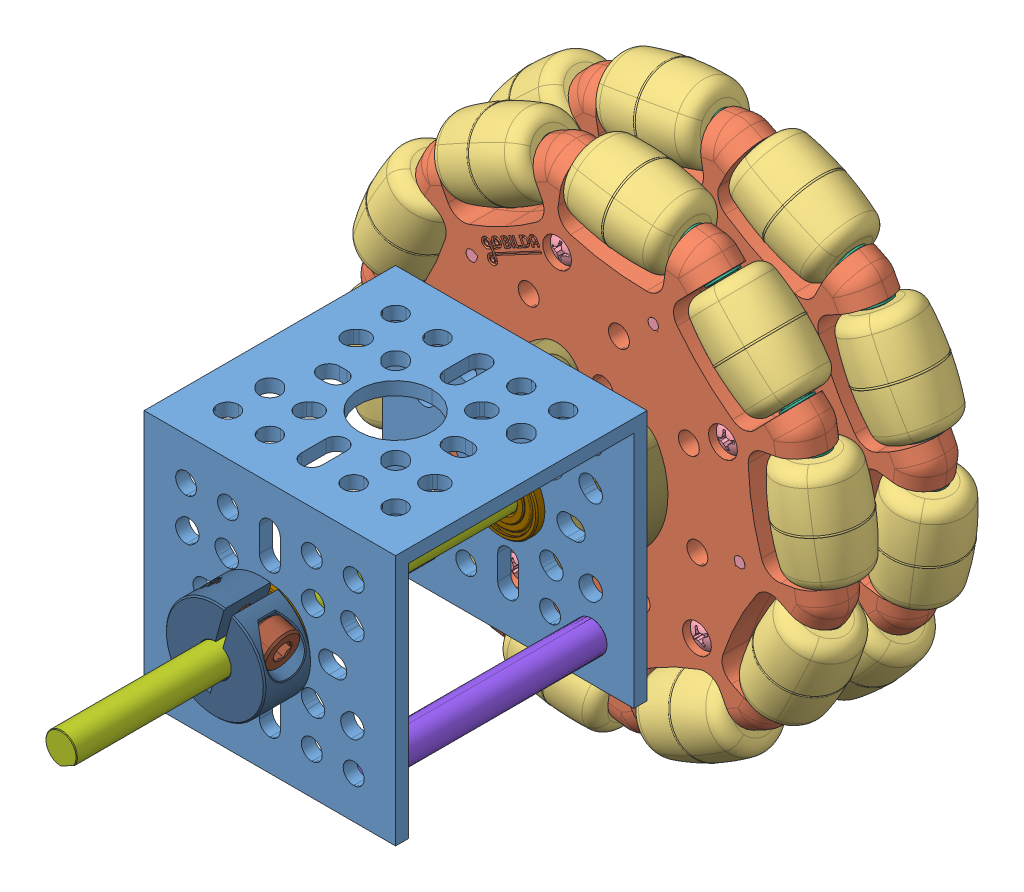
SolidWorks assembly Assemblage7, configuration Défaut. Lengths in mm.
Overall size (132.59 132.59 134.08).
108 component instances, 14 part files, 25 mates.
Components (placement in the parent):
- 1120-0001-0048 u1-1: 1120-0001-0048 u1 [Défaut] at (-19.9494 20.1498 48) x (0 0 1) z (0 1 0) size (48 48 48)
- 3604-0014-0096 assembly-1: 3604-0014-0096 assembly [Défaut] at (32.1351 -34.8102 -33.9164) x (0.468016 -0.88372 0) z (-0.88372 -0.468016 0) size (103.42 20.4 102.56)
  - 3604-0014-0096 assembly.STEP-1: 3604-0014-0096 assembly.STEP [Défaut] at origin size (103.42 20.4 102.56)
    - 3604-0014-0096 wheel half.STEP-1: 3604-0014-0096 wheel half.STEP [Défaut] at (-42.7133 16.9164 9.1591) size (92.38 5.01 87.87)
    - 595671 omni wheel roller.STEP-1: 595671 omni wheel roller.STEP [Défaut] at (-66.8586 21.9164 42.3923) x (0.345492 -0.809017 -0.475528) z (-0.809017 0 -0.587785) size (14.61 14.61 19.05)
    - 364 omni wheel screw_99461A110.STEP-1: 364 omni wheel screw_99461A110.STEP [Défaut] at (-66.9838 22.9164 26.7926) x (-0.972951 0 0.231012) z (0 -1 0) size (5.22 5.22 9.61)
    - 3604-0014-0096 shaft.STEP-1: 3604-0014-0096 shaft.STEP [Défaut] at (-77.1615 21.9164 34.9068) x (0.587659 0.020713 -0.808843) z (0.012175 -0.999785 -0.016757) size (3.17 25.47 3.17)
    - 595671 omni wheel bushing.STEP-1: 595671 omni wheel bushing.STEP [Défaut] at (-66.8586 21.9164 42.3923) x (-0.041473 -0.997508 0.057082) z (-0.809017 0 -0.587785) size (5.61 5.61 20.15)
    - 364 omni wheel screw_99461A110.STEP-2: 364 omni wheel screw_99461A110.STEP [Défaut] at (-66.9838 22.9164 -8.4745) x (-0.520363 0 -0.853945) z (0 -1 0) size (5.22 5.22 9.61)
    - 364 omni wheel screw_99461A110.STEP-3: 364 omni wheel screw_99461A110.STEP [Défaut] at (-33.4428 22.9164 -19.3726) x (0.651349 0 -0.758779) z (0 -1 0) size (5.22 5.22 9.61)
    - 364 omni wheel screw_99461A110.STEP-4: 364 omni wheel screw_99461A110.STEP [Défaut] at (-12.7133 22.9164 9.1591) x (0.922919 0 0.384994) z (0 -1 0) size (5.22 5.22 9.61)
    - 364 omni wheel screw_99461A110.STEP-5: 364 omni wheel screw_99461A110.STEP [Défaut] at (-33.4428 22.9164 37.6908) x (-0.080953 0 0.996718) z (0 -1 0) size (5.22 5.22 9.61)
    - 3604-0014-0096 shaft.STEP-2: 3604-0014-0096 shaft.STEP [Défaut] at (-85.7166 21.9164 9.7413) x (0.950852 0.020713 -0.308951) z (0.019699 -0.999785 -0.006401) size (3.17 25.47 3.17)
    - 3604-0014-0096 shaft.STEP-3: 3604-0014-0096 shaft.STEP [Défaut] at (-77.846 21.9164 -15.6466) x (0.950852 0.020713 0.308951) z (0.019699 -0.999785 0.006401) size (3.17 25.47 3.17)
    - 3604-0014-0096 shaft.STEP-4: 3604-0014-0096 shaft.STEP [Défaut] at (-56.5558 21.9164 -31.5596) x (0.587659 0.020713 0.808843) z (0.012175 -0.999785 0.016757) size (3.17 25.47 3.17)
    - 3604-0014-0096 shaft.STEP-5: 3604-0014-0096 shaft.STEP [Défaut] at (-29.9783 21.9164 -31.9195) x (0 0.020713 0.999785) z (0 -0.999785 0.020713) size (3.17 25.47 3.17)
    - 3604-0014-0096 shaft.STEP-6: 3604-0014-0096 shaft.STEP [Défaut] at (-8.2651 21.9164 -16.5887) x (-0.587659 0.020713 0.808843) z (-0.012175 -0.999785 0.016757) size (3.17 25.47 3.17)
    - 3604-0014-0096 shaft.STEP-7: 3604-0014-0096 shaft.STEP [Défaut] at (0.29 21.9164 8.5768) x (-0.950852 0.020713 0.308951) z (-0.019699 -0.999785 0.006401) size (3.17 25.47 3.17)
    - 3604-0014-0096 shaft.STEP-8: 3604-0014-0096 shaft.STEP [Défaut] at (-7.5806 21.9164 33.9647) x (-0.950852 0.020713 -0.308951) z (-0.019699 -0.999785 -0.006401) size (3.17 25.47 3.17)
    - 3604-0014-0096 shaft.STEP-9: 3604-0014-0096 shaft.STEP [Défaut] at (-28.8708 21.9164 49.8777) x (-0.587659 0.020713 -0.808843) z (-0.012175 -0.999785 -0.016757) size (3.17 25.47 3.17)
    - 3604-0014-0096 shaft.STEP-10: 3604-0014-0096 shaft.STEP [Défaut] at (-55.4483 21.9164 50.2376) x (0 0.020713 -0.999785) z (0 -0.999785 -0.020713) size (3.17 25.47 3.17)
    - 595671 omni wheel bushing.STEP-2: 595671 omni wheel bushing.STEP [Défaut] at (-81.7813 21.9164 21.853) x (-0.067104 -0.997508 0.021803) z (-0.309017 0 -0.951057) size (5.61 5.61 20.15)
    - 595671 omni wheel bushing.STEP-3: 595671 omni wheel bushing.STEP [Défaut] at (-81.7813 21.9164 -3.5349) x (-0.067104 -0.997508 -0.021803) z (0.309017 0 -0.951057) size (5.61 5.61 20.15)
    - 595671 omni wheel bushing.STEP-4: 595671 omni wheel bushing.STEP [Défaut] at (-66.8586 21.9164 -24.0742) x (-0.041473 -0.997508 -0.057082) z (0.809017 0 -0.587785) size (5.61 5.61 20.15)
    - 595671 omni wheel bushing.STEP-5: 595671 omni wheel bushing.STEP [Défaut] at (-42.7133 21.9164 -31.9195) x (0 -0.997508 -0.070558) z (1 0 0) size (5.61 5.61 20.15)
    - 595671 omni wheel bushing.STEP-6: 595671 omni wheel bushing.STEP [Défaut] at (-18.5679 21.9164 -24.0742) x (0.041473 -0.997508 -0.057082) z (0.809017 0 0.587785) size (5.61 5.61 20.15)
    - 595671 omni wheel bushing.STEP-7: 595671 omni wheel bushing.STEP [Défaut] at (-3.6453 21.9164 -3.5349) x (0.067104 -0.997508 -0.021803) z (0.309017 0 0.951057) size (5.61 5.61 20.15)
    - 595671 omni wheel bushing.STEP-8: 595671 omni wheel bushing.STEP [Défaut] at (-3.6453 21.9164 21.853) x (0.067104 -0.997508 0.021803) z (-0.309017 0 0.951057) size (5.61 5.61 20.15)
    - 595671 omni wheel bushing.STEP-9: 595671 omni wheel bushing.STEP [Défaut] at (-18.5679 21.9164 42.3923) x (0.041473 -0.997508 0.057082) z (-0.809017 0 0.587785) size (5.61 5.61 20.15)
    - 595671 omni wheel bushing.STEP-10: 595671 omni wheel bushing.STEP [Défaut] at (-42.7133 21.9164 50.2376) x (0 -0.997508 0.070558) z (-1 0 0) size (5.61 5.61 20.15)
    - 595671 omni wheel roller.STEP-2: 595671 omni wheel roller.STEP [Défaut] at (-81.7813 21.9164 21.853) x (0.559017 -0.809017 -0.181636) z (-0.309017 0 -0.951057) size (14.61 14.61 19.05)
    - 595671 omni wheel roller.STEP-3: 595671 omni wheel roller.STEP [Défaut] at (-81.7813 21.9164 -3.5349) x (0.559017 -0.809017 0.181636) z (0.309017 0 -0.951057) size (14.61 14.61 19.05)
    - 595671 omni wheel roller.STEP-4: 595671 omni wheel roller.STEP [Défaut] at (-66.8586 21.9164 -24.0742) x (0.345492 -0.809017 0.475528) z (0.809017 0 -0.587785) size (14.61 14.61 19.05)
    - 595671 omni wheel roller.STEP-5: 595671 omni wheel roller.STEP [Défaut] at (-42.7133 21.9164 -31.9195) x (0 -0.809017 0.587785) z (1 0 0) size (14.61 14.61 19.05)
    - 595671 omni wheel roller.STEP-6: 595671 omni wheel roller.STEP [Défaut] at (-18.5679 21.9164 -24.0742) x (-0.345492 -0.809017 0.475528) z (0.809017 0 0.587785) size (14.61 14.61 19.05)
    - 595671 omni wheel roller.STEP-7: 595671 omni wheel roller.STEP [Défaut] at (-3.6453 21.9164 -3.5349) x (-0.559017 -0.809017 0.181636) z (0.309017 0 0.951057) size (14.61 14.61 19.05)
    - 595671 omni wheel roller.STEP-8: 595671 omni wheel roller.STEP [Défaut] at (-3.6453 21.9164 21.853) x (-0.559017 -0.809017 -0.181636) z (-0.309017 0 0.951057) size (14.61 14.61 19.05)
    - 595671 omni wheel roller.STEP-9: 595671 omni wheel roller.STEP [Défaut] at (-18.5679 21.9164 42.3923) x (-0.345492 -0.809017 -0.475528) z (-0.809017 0 0.587785) size (14.61 14.61 19.05)
    - 595671 omni wheel roller.STEP-10: 595671 omni wheel roller.STEP [Défaut] at (-42.7133 21.9164 50.2376) x (0 -0.809017 -0.587785) z (-1 0 0) size (14.61 14.61 19.05)
    - 3604-0014-0096 wheel half.STEP-2: 3604-0014-0096 wheel half.STEP [Défaut] at (-42.7133 26.9164 9.1591) x (-1 0 0) z (0 0 1) size (92.38 5.01 87.87)
    - 364 omni wheel screw_99461A110.STEP-6: 364 omni wheel screw_99461A110.STEP [Défaut] at (-51.9838 20.9164 37.6908) x (-0.514694 0 0.857374) z (0 1 0) size (5.22 5.22 9.61)
    - 364 omni wheel screw_99461A110.STEP-7: 364 omni wheel screw_99461A110.STEP [Défaut] at (-18.4428 20.9164 26.7926) x (0.656361 0 0.754447) z (0 1 0) size (5.22 5.22 9.61)
    - 364 omni wheel screw_99461A110.STEP-8: 364 omni wheel screw_99461A110.STEP [Défaut] at (-18.4428 20.9164 -8.4745) x (0.920348 0 -0.3911) z (0 1 0) size (5.22 5.22 9.61)
    - 364 omni wheel screw_99461A110.STEP-9: 364 omni wheel screw_99461A110.STEP [Défaut] at (-51.9838 20.9164 -19.3726) x (-0.087555 0 -0.99616) z (0 1 0) size (5.22 5.22 9.61)
    - 364 omni wheel screw_99461A110.STEP-10: 364 omni wheel screw_99461A110.STEP [Défaut] at (-72.7133 20.9164 9.1591) x (-0.97446 0 -0.22456) z (0 1 0) size (5.22 5.22 9.61)
- 3604-0014-0096 assembly-2: 3604-0014-0096 assembly [Défaut] at (-29.4094 -29.4347 -14.9164) x (-0.88372 -0.468016 0) z (-0.468016 0.88372 0) size (103.42 20.4 102.56)
  - 3604-0014-0096 assembly.STEP-1: 3604-0014-0096 assembly.STEP [Défaut] at origin size (103.42 20.4 102.56)
    - 3604-0014-0096 wheel half.STEP-1: 3604-0014-0096 wheel half.STEP [Défaut] at (-42.7133 16.9164 9.1591) size (92.38 5.01 87.87)
    - 595671 omni wheel roller.STEP-1: 595671 omni wheel roller.STEP [Défaut] at (-66.8586 21.9164 42.3923) x (0.345492 -0.809017 -0.475528) z (-0.809017 0 -0.587785) size (14.61 14.61 19.05)
    - 364 omni wheel screw_99461A110.STEP-1: 364 omni wheel screw_99461A110.STEP [Défaut] at (-66.9838 22.9164 26.7926) x (-0.972951 0 0.231012) z (0 -1 0) size (5.22 5.22 9.61)
    - 3604-0014-0096 shaft.STEP-1: 3604-0014-0096 shaft.STEP [Défaut] at (-77.1615 21.9164 34.9068) x (0.587659 0.020713 -0.808843) z (0.012175 -0.999785 -0.016757) size (3.17 25.47 3.17)
    - 595671 omni wheel bushing.STEP-1: 595671 omni wheel bushing.STEP [Défaut] at (-66.8586 21.9164 42.3923) x (-0.041473 -0.997508 0.057082) z (-0.809017 0 -0.587785) size (5.61 5.61 20.15)
    - 364 omni wheel screw_99461A110.STEP-2: 364 omni wheel screw_99461A110.STEP [Défaut] at (-66.9838 22.9164 -8.4745) x (-0.520363 0 -0.853945) z (0 -1 0) size (5.22 5.22 9.61)
    - 364 omni wheel screw_99461A110.STEP-3: 364 omni wheel screw_99461A110.STEP [Défaut] at (-33.4428 22.9164 -19.3726) x (0.651349 0 -0.758779) z (0 -1 0) size (5.22 5.22 9.61)
    - 364 omni wheel screw_99461A110.STEP-4: 364 omni wheel screw_99461A110.STEP [Défaut] at (-12.7133 22.9164 9.1591) x (0.922919 0 0.384994) z (0 -1 0) size (5.22 5.22 9.61)
    - 364 omni wheel screw_99461A110.STEP-5: 364 omni wheel screw_99461A110.STEP [Défaut] at (-33.4428 22.9164 37.6908) x (-0.080953 0 0.996718) z (0 -1 0) size (5.22 5.22 9.61)
    - 3604-0014-0096 shaft.STEP-2: 3604-0014-0096 shaft.STEP [Défaut] at (-85.7166 21.9164 9.7413) x (0.950852 0.020713 -0.308951) z (0.019699 -0.999785 -0.006401) size (3.17 25.47 3.17)
    - 3604-0014-0096 shaft.STEP-3: 3604-0014-0096 shaft.STEP [Défaut] at (-77.846 21.9164 -15.6466) x (0.950852 0.020713 0.308951) z (0.019699 -0.999785 0.006401) size (3.17 25.47 3.17)
    - 3604-0014-0096 shaft.STEP-4: 3604-0014-0096 shaft.STEP [Défaut] at (-56.5558 21.9164 -31.5596) x (0.587659 0.020713 0.808843) z (0.012175 -0.999785 0.016757) size (3.17 25.47 3.17)
    - 3604-0014-0096 shaft.STEP-5: 3604-0014-0096 shaft.STEP [Défaut] at (-29.9783 21.9164 -31.9195) x (0 0.020713 0.999785) z (0 -0.999785 0.020713) size (3.17 25.47 3.17)
    - 3604-0014-0096 shaft.STEP-6: 3604-0014-0096 shaft.STEP [Défaut] at (-8.2651 21.9164 -16.5887) x (-0.587659 0.020713 0.808843) z (-0.012175 -0.999785 0.016757) size (3.17 25.47 3.17)
    - 3604-0014-0096 shaft.STEP-7: 3604-0014-0096 shaft.STEP [Défaut] at (0.29 21.9164 8.5768) x (-0.950852 0.020713 0.308951) z (-0.019699 -0.999785 0.006401) size (3.17 25.47 3.17)
    - 3604-0014-0096 shaft.STEP-8: 3604-0014-0096 shaft.STEP [Défaut] at (-7.5806 21.9164 33.9647) x (-0.950852 0.020713 -0.308951) z (-0.019699 -0.999785 -0.006401) size (3.17 25.47 3.17)
    - 3604-0014-0096 shaft.STEP-9: 3604-0014-0096 shaft.STEP [Défaut] at (-28.8708 21.9164 49.8777) x (-0.587659 0.020713 -0.808843) z (-0.012175 -0.999785 -0.016757) size (3.17 25.47 3.17)
    - 3604-0014-0096 shaft.STEP-10: 3604-0014-0096 shaft.STEP [Défaut] at (-55.4483 21.9164 50.2376) x (0 0.020713 -0.999785) z (0 -0.999785 -0.020713) size (3.17 25.47 3.17)
    - 595671 omni wheel bushing.STEP-2: 595671 omni wheel bushing.STEP [Défaut] at (-81.7813 21.9164 21.853) x (-0.067104 -0.997508 0.021803) z (-0.309017 0 -0.951057) size (5.61 5.61 20.15)
    - 595671 omni wheel bushing.STEP-3: 595671 omni wheel bushing.STEP [Défaut] at (-81.7813 21.9164 -3.5349) x (-0.067104 -0.997508 -0.021803) z (0.309017 0 -0.951057) size (5.61 5.61 20.15)
    - 595671 omni wheel bushing.STEP-4: 595671 omni wheel bushing.STEP [Défaut] at (-66.8586 21.9164 -24.0742) x (-0.041473 -0.997508 -0.057082) z (0.809017 0 -0.587785) size (5.61 5.61 20.15)
    - 595671 omni wheel bushing.STEP-5: 595671 omni wheel bushing.STEP [Défaut] at (-42.7133 21.9164 -31.9195) x (0 -0.997508 -0.070558) z (1 0 0) size (5.61 5.61 20.15)
    - 595671 omni wheel bushing.STEP-6: 595671 omni wheel bushing.STEP [Défaut] at (-18.5679 21.9164 -24.0742) x (0.041473 -0.997508 -0.057082) z (0.809017 0 0.587785) size (5.61 5.61 20.15)
    - 595671 omni wheel bushing.STEP-7: 595671 omni wheel bushing.STEP [Défaut] at (-3.6453 21.9164 -3.5349) x (0.067104 -0.997508 -0.021803) z (0.309017 0 0.951057) size (5.61 5.61 20.15)
    - 595671 omni wheel bushing.STEP-8: 595671 omni wheel bushing.STEP [Défaut] at (-3.6453 21.9164 21.853) x (0.067104 -0.997508 0.021803) z (-0.309017 0 0.951057) size (5.61 5.61 20.15)
    - 595671 omni wheel bushing.STEP-9: 595671 omni wheel bushing.STEP [Défaut] at (-18.5679 21.9164 42.3923) x (0.041473 -0.997508 0.057082) z (-0.809017 0 0.587785) size (5.61 5.61 20.15)
    - 595671 omni wheel bushing.STEP-10: 595671 omni wheel bushing.STEP [Défaut] at (-42.7133 21.9164 50.2376) x (0 -0.997508 0.070558) z (-1 0 0) size (5.61 5.61 20.15)
    - 595671 omni wheel roller.STEP-2: 595671 omni wheel roller.STEP [Défaut] at (-81.7813 21.9164 21.853) x (0.559017 -0.809017 -0.181636) z (-0.309017 0 -0.951057) size (14.61 14.61 19.05)
    - 595671 omni wheel roller.STEP-3: 595671 omni wheel roller.STEP [Défaut] at (-81.7813 21.9164 -3.5349) x (0.559017 -0.809017 0.181636) z (0.309017 0 -0.951057) size (14.61 14.61 19.05)
    - 595671 omni wheel roller.STEP-4: 595671 omni wheel roller.STEP [Défaut] at (-66.8586 21.9164 -24.0742) x (0.345492 -0.809017 0.475528) z (0.809017 0 -0.587785) size (14.61 14.61 19.05)
    - 595671 omni wheel roller.STEP-5: 595671 omni wheel roller.STEP [Défaut] at (-42.7133 21.9164 -31.9195) x (0 -0.809017 0.587785) z (1 0 0) size (14.61 14.61 19.05)
    - 595671 omni wheel roller.STEP-6: 595671 omni wheel roller.STEP [Défaut] at (-18.5679 21.9164 -24.0742) x (-0.345492 -0.809017 0.475528) z (0.809017 0 0.587785) size (14.61 14.61 19.05)
    - 595671 omni wheel roller.STEP-7: 595671 omni wheel roller.STEP [Défaut] at (-3.6453 21.9164 -3.5349) x (-0.559017 -0.809017 0.181636) z (0.309017 0 0.951057) size (14.61 14.61 19.05)
    - 595671 omni wheel roller.STEP-8: 595671 omni wheel roller.STEP [Défaut] at (-3.6453 21.9164 21.853) x (-0.559017 -0.809017 -0.181636) z (-0.309017 0 0.951057) size (14.61 14.61 19.05)
    - 595671 omni wheel roller.STEP-9: 595671 omni wheel roller.STEP [Défaut] at (-18.5679 21.9164 42.3923) x (-0.345492 -0.809017 -0.475528) z (-0.809017 0 0.587785) size (14.61 14.61 19.05)
    - 595671 omni wheel roller.STEP-10: 595671 omni wheel roller.STEP [Défaut] at (-42.7133 21.9164 50.2376) x (0 -0.809017 -0.587785) z (-1 0 0) size (14.61 14.61 19.05)
    - 3604-0014-0096 wheel half.STEP-2: 3604-0014-0096 wheel half.STEP [Défaut] at (-42.7133 26.9164 9.1591) x (-1 0 0) z (0 0 1) size (92.38 5.01 87.87)
    - 364 omni wheel screw_99461A110.STEP-6: 364 omni wheel screw_99461A110.STEP [Défaut] at (-51.9838 20.9164 37.6908) x (-0.514694 0 0.857374) z (0 1 0) size (5.22 5.22 9.61)
    - 364 omni wheel screw_99461A110.STEP-7: 364 omni wheel screw_99461A110.STEP [Défaut] at (-18.4428 20.9164 26.7926) x (0.656361 0 0.754447) z (0 1 0) size (5.22 5.22 9.61)
    - 364 omni wheel screw_99461A110.STEP-8: 364 omni wheel screw_99461A110.STEP [Défaut] at (-18.4428 20.9164 -8.4745) x (0.920348 0 -0.3911) z (0 1 0) size (5.22 5.22 9.61)
    - 364 omni wheel screw_99461A110.STEP-9: 364 omni wheel screw_99461A110.STEP [Défaut] at (-51.9838 20.9164 -19.3726) x (-0.087555 0 -0.99616) z (0 1 0) size (5.22 5.22 9.61)
    - 364 omni wheel screw_99461A110.STEP-10: 364 omni wheel screw_99461A110.STEP [Défaut] at (-72.7133 20.9164 9.1591) x (-0.97446 0 -0.22456) z (0 1 0) size (5.22 5.22 9.61)
- 2101-0006-0100 essieuCourt-1: 2101-0006-0100 essieuCourt [Défaut] at (4.0506 -1.3502 11.875) x (-0.88372 -0.468016 0) z (-0.468016 0.88372 0) size (6 100 5.5)
- 1501-0006-0430 renfort-1: 1501-0006-0430 renfort [Défaut] at (-11.9494 -17.3502 48) x (0 1 0) z (1 0 0) size (5.95 43.01 5.95)
- 1501-0006-0430 renfort-2: 1501-0006-0430 renfort [Défaut] at (20.0506 -17.3502 48) x (1 0 0) z (0 -1 0) size (5.95 43.01 5.95)
- 1611-0514-0006-1: 1611-0514-0006 [Défaut] at (4.0506 -1.3502 28) x (-0.582956 0.812503 0) z (-0.812503 -0.582956 0) size (15 5 15)
- 1611-0514-0006-2: 1611-0514-0006 [Défaut] at (4.0506 -1.3502 68) x (0.993873 0.110524 0) z (0.110524 -0.993873 0) size (15 5 15)
- 2910-0919-0006 assembly collet-1: 2910-0919-0006 assembly collet [Défaut] at (-2.1504 -36.0754 -1.9796) x (-0.621578 -0.783352 0) z (-0.783352 0.621578 0) size (19 9.89 19.83)
  - 2910-0919-0006 assembly.STEP-1: 2910-0919-0006 assembly.STEP [Défaut] at origin size (19 9.89 19.83)
    - 2910-0919-0006.STEP-1: 2910-0919-0006.STEP [Défaut] at (-31.0565 -0.5204 16.7268) size (19 9.5 18.97)
    - 2800-0004-0010_90128A207.STEP-1: 2800-0004-0010_90128A207.STEP [Défaut] at (-24.2865 -0.5204 11.2868) x (0 -0.807243 -0.59022) z (1 0 0) size (7 7 14.01)
- 1309-0016-1006 assembly-1: 1309-0016-1006 assembly [Défaut] at (-1.8519 -18.5782 7.2264) x (-0.293947 -0.955822 0) z (0 0 1) size (28.36 32 10.95)
  - 1309-0016-1006 assembly.STEP-1: 1309-0016-1006 assembly.STEP [Défaut] at origin size (28.36 32 10.95)
    - 1309-0016-1006.STEP-1: 1309-0016-1006.STEP [Défaut] at (-18.2019 0.5776 8.7736) size (25.38 32 10)
    - 2800-0004-0014_90128A207.STEP-1: 2800-0004-0014_90128A207.STEP [Défaut] at (-16.149 11.6963 8.7736) x (0.5 -0.5 -0.707107) z (0.707107 0.707107 0) size (7 7 18.01)
    - 2800-0004-0014_90128A207.STEP-2: 2800-0004-0014_90128A207.STEP [Défaut] at (-20.2547 -10.5411 8.7736) x (-0.5 0.5 -0.707107) z (-0.707107 -0.707107 0) size (7 7 18.01)
- 2910-0919-0006 assembly collet-2: 2910-0919-0006 assembly collet [Défaut] at (-21.4149 23.0588 77.4796) x (-0.963724 0.266899 0) z (-0.266899 -0.963724 0) size (19 9.89 19.83)
  - 2910-0919-0006 assembly.STEP-1: 2910-0919-0006 assembly.STEP [Défaut] at origin size (19 9.89 19.83)
    - 2910-0919-0006.STEP-1: 2910-0919-0006.STEP [Défaut] at (-31.0565 -0.5204 16.7268) size (19 9.5 18.97)
    - 2800-0004-0010_90128A207.STEP-1: 2800-0004-0010_90128A207.STEP [Défaut] at (-24.2865 -0.5204 11.2868) x (0 -0.807243 -0.59022) z (1 0 0) size (7 7 14.01)
- 2807-0609-1000-1: 2807-0609-1000 [Défaut] at (4.0506 -1.3502 22) x (1 0 0) z (0 -1 0) size (9 1 9)
Mates (geometry in assembly coordinates):
- Coaxiale2: concentric: cylinder of 3604-0014-0096 assembly-1/3604-0014-0096 assembly.STEP-1/3604-0014-0096 wheel half.STEP-1 through (4.0506 -1.3502 -12) axis (0 0 -1) radius 7; cylinder of 2101-0006-0100 essieuCourt-1 through (4.0506 -1.3502 111.875) axis (0 0 -1) radius 3
- Coaxiale3: concentric: cylinder of 1120-0001-0048 u1-1 through (4.0506 -1.3502 34) axis (0 0 -1) radius 7; cylinder of 2101-0006-0100 essieuCourt-1 through (4.0506 -1.3502 111.875) axis (0 0 -1) radius 3
- Coaxiale4: concentric: cylinder of 3604-0014-0096 assembly-2/3604-0014-0096 assembly.STEP-1/3604-0014-0096 wheel half.STEP-1 through (4.0506 -1.3502 7) axis (0 0 -1) radius 7; cylinder of 2101-0006-0100 essieuCourt-1 through (4.0506 -1.3502 111.875) axis (0 0 -1) radius 3
- Coaxiale5: concentric: cylinder of 3604-0014-0096 assembly-1/3604-0014-0096 assembly.STEP-1/3604-0014-0096 wheel half.STEP-1 through (-7.4193 2.1772 -12) axis (0 0 -1) radius 2; cylinder of 3604-0014-0096 assembly-2/3604-0014-0096 assembly.STEP-1/3604-0014-0096 wheel half.STEP-1 through (-7.4193 2.1772 7) axis (0 0 -1) radius 2
- Coaxiale7: concentric: cylinder of 2101-0006-0100 essieuCourt-1 through (4.0506 -1.3502 111.875) axis (0 0 -1) radius 3; cylinder of 2910-0919-0006 assembly collet-1/2910-0919-0006 assembly.STEP-1/2910-0919-0006.STEP-1 through (4.0506 -1.3502 2) axis (0 0 -1) radius 3
- Coïncidente1: coincident: plane of 3604-0014-0096 assembly-1/3604-0014-0096 assembly.STEP-1/3604-0014-0096 wheel half.STEP-2 through (4.0506 -1.3502 -7) normal (0 0 1); plane of 2910-0919-0006 assembly collet-1/2910-0919-0006 assembly.STEP-1/2910-0919-0006.STEP-1 through (4.0506 -1.3502 -7) normal (0 0 -1)
- Coïncidente2: coincident: plane of 3604-0014-0096 assembly-2/3604-0014-0096 assembly.STEP-1/3604-0014-0096 wheel half.STEP-1 through (4.0506 -1.3502 2) normal (0 0 -1); plane of 2910-0919-0006 assembly collet-1/2910-0919-0006 assembly.STEP-1/2910-0919-0006.STEP-1 through (4.0506 -1.3502 2) normal (0 0 1)
- Coaxiale8: concentric: cylinder of 2101-0006-0100 essieuCourt-1 through (4.0506 -1.3502 111.875) axis (0 0 -1) radius 3; cylinder of 1611-0514-0006-1 through (4.0506 -1.3502 28) axis (0 0 -1) radius 3
- Coaxiale9: concentric: cylinder of 2101-0006-0100 essieuCourt-1 through (4.0506 -1.3502 111.875) axis (0 0 -1) radius 3; cylinder of 1309-0016-1006 assembly-1/1309-0016-1006 assembly.STEP-1/1309-0016-1006.STEP-1 through (4.0506 -1.3502 11.7495) axis (0 0 1) radius 3
- Parallèle1: parallel: plane of 2101-0006-0100 essieuCourt-1 through (5.2206 -3.5595 111.875) normal (0.468016 -0.88372 0); line of 1309-0016-1006 assembly-1/1309-0016-1006 assembly.STEP-1/1309-0016-1006.STEP-1 through (6.7031 -2.7518 22) axis (-0.88372 -0.468016 0)
- Coïncidente4: coincident: circle of 2101-0006-0100 essieuCourt-1; plane of 1309-0016-1006 assembly-1/1309-0016-1006 assembly.STEP-1/1309-0016-1006.STEP-1 through (4.0506 -1.3502 12) normal (0 0 -1)
- Coïncidente5: coincident: plane of 3604-0014-0096 assembly-2/3604-0014-0096 assembly.STEP-1/3604-0014-0096 wheel half.STEP-2 through (4.0506 -1.3502 12) normal (0 0 1); plane of 1309-0016-1006 assembly-1/1309-0016-1006 assembly.STEP-1/1309-0016-1006.STEP-1 through (4.0506 -1.3502 12) normal (0 0 -1)
- Coïncidente6: coincident: plane of 1120-0001-0048 u1-1 through (28.0506 -25.3502 24) normal (0 0 -1); plane of 1611-0514-0006-1 through (4.0506 -1.3502 24) normal (0 0 1)
- Coaxiale10: concentric: cylinder of 2101-0006-0100 essieuCourt-1 through (4.0506 -1.3502 111.875) axis (0 0 -1) radius 3; cylinder of 2807-0609-1000-1 through (4.0506 -1.3502 23) axis (0 0 -1) radius 3
- Coïncidente7: coincident: plane of 1611-0514-0006-1 through (4.0506 -1.3502 23) normal (0 0 -1); plane of 2807-0609-1000-1 through (4.0506 -1.3502 23) normal (0 0 1)
- Coïncidente8: coincident: plane of 1309-0016-1006 assembly-1/1309-0016-1006 assembly.STEP-1/1309-0016-1006.STEP-1 through (4.0506 -1.3502 22) normal (0 0 1); plane of 2807-0609-1000-1 through (4.0506 -1.3502 22) normal (0 0 -1)
- Coaxiale11: concentric: cylinder of 2101-0006-0100 essieuCourt-1 through (4.0506 -1.3502 111.875) axis (0 0 -1) radius 3; cylinder of 1611-0514-0006-2 through (4.0506 -1.3502 68) axis (0 0 1) radius 3
- Coïncidente9: coincident: plane of 1120-0001-0048 u1-1 through (28.0506 -25.3502 72) normal (0 0 1); plane of 1611-0514-0006-2 through (4.0506 -1.3502 72) normal (0 0 -1)
- Coaxiale15: concentric: circle of 3604-0014-0096 assembly-1/3604-0014-0096 assembly.STEP-1/3604-0014-0096 wheel half.STEP-1; circle of 1309-0016-1006 assembly-1/1309-0016-1006 assembly.STEP-1/1309-0016-1006.STEP-1
- Coaxiale17: concentric: cylinder of 2101-0006-0100 essieuCourt-1 through (4.0506 -1.3502 111.875) axis (0 0 -1) radius 3; cylinder of 2910-0919-0006 assembly collet-2/2910-0919-0006 assembly.STEP-1/2910-0919-0006.STEP-1 through (4.0506 -1.3502 73.5) axis (0 0 1) radius 3
- Coïncidente12: coincident: plane of 1611-0514-0006-2 through (4.0506 -1.3502 73) normal (0 0 1); plane of 2910-0919-0006 assembly collet-2/2910-0919-0006 assembly.STEP-1/2910-0919-0006.STEP-1 through (4.0506 -1.3502 73) normal (0 0 -1)
- Coïncidente13: coincident: plane of 1120-0001-0048 u1-1 through (28.0506 20.1498 69.5) normal (0 0 -1); plane of 1501-0006-0430 renfort-2 through (20.0506 -17.3502 69.5) normal (0 0 1)
- Coaxiale18: concentric: cylinder of 1120-0001-0048 u1-1 through (20.0506 -17.3502 62) axis (0 0 1) radius 2; cylinder of 1501-0006-0430 renfort-2 through (20.0506 -17.3502 69.5) axis (0 0 -1) radius 2.975
- Coïncidente14: coincident: plane of 1120-0001-0048 u1-1 through (28.0506 20.1498 69.5) normal (0 0 -1); plane of 1501-0006-0430 renfort-1 through (-11.9494 -17.3502 69.5) normal (0 0 1)
- Coaxiale19: concentric: cylinder of 1120-0001-0048 u1-1 through (-11.9494 -17.3502 62) axis (0 0 1) radius 2; cylinder of 1501-0006-0430 renfort-1 through (-11.9494 -17.3502 69.5) axis (0 0 -1) radius 2.975
